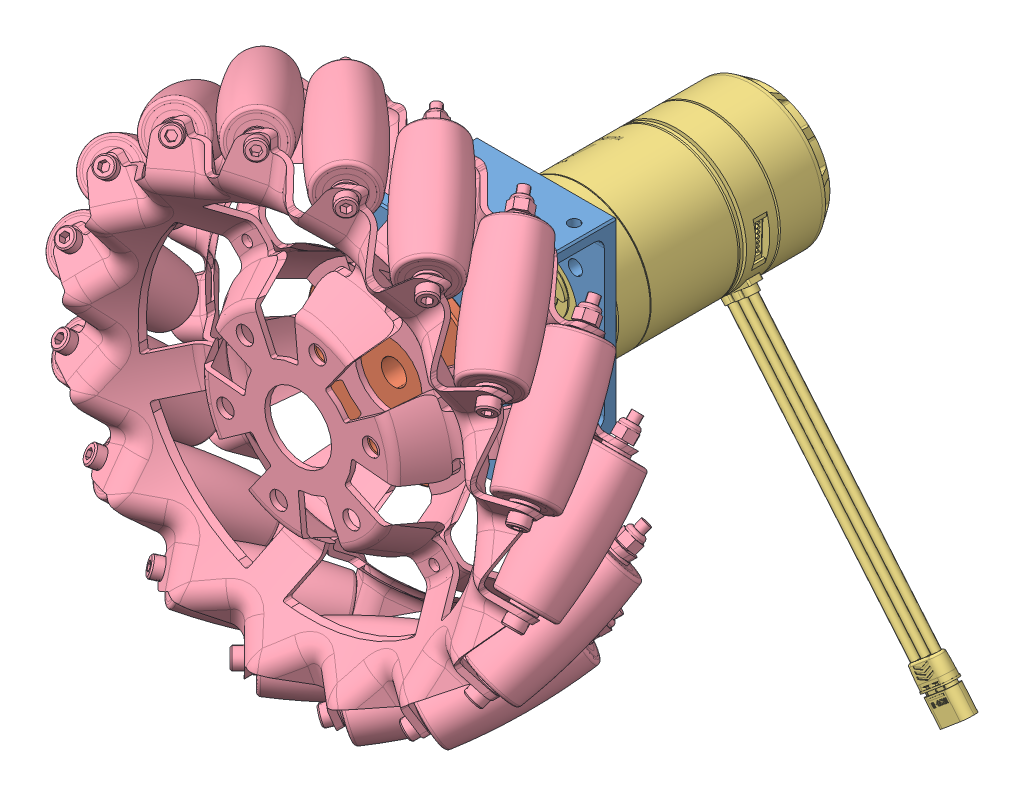
SolidWorks assembly 麦轮电机总装右, configuration 默认. Lengths in mm.
Overall size (224.64 231.76 154.77).
5 component instances, 4 part files, 3 mates.
Components (placement in the parent):
- 3508-1: 3508 [Default] at (20.407 2.6404 90.2458) size (124.33 157.68 116.9)
  - 电机座Z80123-1: 电机座Z80123 [默认] at (-77.6885 26.4734 96.0875) size (42 55.4 32)
  - 电机连轴Z80123-1: 电机连轴Z80123 [默认] at (-77.6885 26.4734 125.8875) x (0.707107 -0.707107 0) z (0.707107 0.707107 0) size (55 37.5 55)
  - M3508直流无刷减速电机-2: M3508直流无刷减速电机 [默认] at (-69.0293 10.2886 -6.3535) x (0.923508 0.383579 0) z (0 0 1) size (63.71 141 98.4)
- 麦轮镂空（右）-1: 麦轮镂空（右） [默认] at (-150.2658 -73.4679 151.1394) x (-0.707107 0.707107 0) z (0.707107 0.707107 0) size (182.09 47.13 182.09)
Mates (geometry in assembly coordinates):
- 同心1: concentric aligned: cylinder of 3508-1/电机连轴Z80123-1 through (-57.2815 29.1138 216.1333) axis (0 0 -1) radius 3.75; cylinder of 麦轮镂空（右）-1 through (-57.2815 29.1138 244.895) axis (0 0 -1) radius 10
- 同心2: concentric aligned: cylinder of 3508-1/电机连轴Z80123-1 through (-73.1914 45.0237 205.1333) axis (0 0 1) radius 2.6; cylinder of 麦轮镂空（右）-1 through (-73.1914 45.0237 242.9723) axis (0 0 1) radius 2.6
- 重合1: coincident anti-aligned: plane of 3508-1/电机连轴Z80123-1 through (-57.2815 29.1138 216.1333) normal (0 0 1); plane of 麦轮镂空（右）-1 through (-52.8331 -16.0519 216.1333) normal (0 0 -1)
